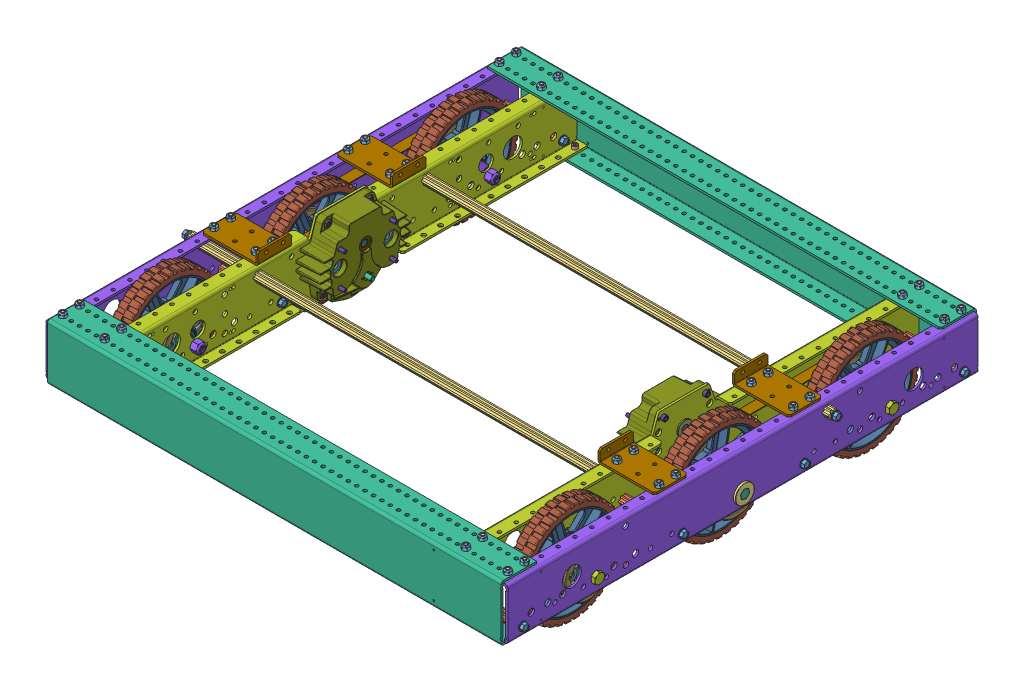
SolidWorks assembly 0 AM14U3 Full Square Drive Base, configuration Default. Lengths in mm.
Overall size (735.08 197.16 719.07).
302 component instances, 35 part files, 0 mates.
Components (placement in the parent):
- AM14U3 Square Half-1: AM14U3 Square Half [Default] at (-83.3124 74.3045 8.4761) size (722.96 197.16 715.14) (flexible)
  - AM14U3 Square Frame Half-1: AM14U3 Square Frame Half [Default] at (326.068 37.2757 -291.2758) size (722.38 116.33 715.14)
    - ThreadRollingScrew_0.25-20x0.75_FHTS 0.25-20-G-0.75-C-1: ThreadRollingScrew_0.25-20x0.75_FHTS 0.25-20-G-0.75-C [Default] at (-600.075 -67.691 639.064) x (-1 0 0) z (0 0.924225 0.381849) size (24.64 12.19 12.19)
    - ThreadRollingScrew_0.25-20x0.75_FHTS 0.25-20-G-0.75-C-2: ThreadRollingScrew_0.25-20x0.75_FHTS 0.25-20-G-0.75-C [Default] at (-600.075 -67.691 -27.94) x (-1 0 0) z (0 0.924225 0.381849) size (24.64 12.19 12.19)
    - ThreadRollingScrew_0.25-20x0.75_FHTS 0.25-20-G-0.75-C-3: ThreadRollingScrew_0.25-20x0.75_FHTS 0.25-20-G-0.75-C [Default] at (-692.15 -67.691 -27.813) size (24.64 12.19 12.19)
    - ThreadRollingScrew_0.25-20x0.75_FHTS 0.25-20-G-0.75-C-4: ThreadRollingScrew_0.25-20x0.75_FHTS 0.25-20-G-0.75-C [Default] at (-603.25 -15.494 178.562) size (24.64 12.19 12.19)
    - ThreadRollingScrew_0.25-20x0.75_FHTS 0.25-20-G-0.75-C-5: ThreadRollingScrew_0.25-20x0.75_FHTS 0.25-20-G-0.75-C [Default] at (-692.15 -67.691 638.937) size (24.64 12.19 12.19)
    - ThreadRollingScrew_0.25-20x0.75_FHTS 0.25-20-G-0.75-C-6: ThreadRollingScrew_0.25-20x0.75_FHTS 0.25-20-G-0.75-C [Default] at (19.05 -15.494 178.562) x (-1 0 0) z (0 0.525103 -0.851039) size (24.64 12.19 12.19)
    - 500Churro_3.375-1: 500Churro_3.375 [Default] at (-603.25 -67.691 -27.813) x (0 -0.866025 0.5) z (-1 0 0) size (14.66 12.7 85.72)
    - 500Churro_3.375-2: 500Churro_3.375 [Default] at (-603.25 -67.691 638.937) x (0 -0.866025 0.5) z (-1 0 0) size (14.66 12.7 85.72)
    - 500Churro_24.25-1: 500Churro_24.25 [Default] at (15.875 -15.494 178.562) x (0 0 -1) z (-1 0 0) size (14.66 12.7 615.95)
    - Screw_SHCS_10-32x0.5_HX-SHCS 0.19-32x1.375x1-C-1: Screw_SHCS_10-32x0.5_HX-SHCS 0.19-32x1.375x1-C [Default] at (-679.45 -11.43 -11.938) x (0 1 0) z (-0.440454 0 0.897775) size (17.53 7.94 7.94)
    - Screw_SHCS_10-32x0.5_HX-SHCS 0.19-32x1.375x1-C-2: Screw_SHCS_10-32x0.5_HX-SHCS 0.19-32x1.375x1-C [Default] at (-679.45 -11.43 -37.338) x (0 1 0) z (-0.063425 0 0.997987) size (17.53 7.94 7.94)
    - Screw_SHCS_10-32x0.5_HX-SHCS 0.19-32x1.375x1-C-3: Screw_SHCS_10-32x0.5_HX-SHCS 0.19-32x1.375x1-C [Default] at (-615.95 -11.43 -37.338) x (0 1 0) z (0 0 1) size (17.53 7.94 7.94)
    - Screw_SHCS_10-32x0.5_HX-SHCS 0.19-32x1.375x1-C-4: Screw_SHCS_10-32x0.5_HX-SHCS 0.19-32x1.375x1-C [Default] at (-615.95 -11.43 -11.938) x (0 1 0) z (0 0 1) size (17.53 7.94 7.94)
    - Screw_SHCS_10-32x0.5_HX-SHCS 0.19-32x1.375x1-C-5: Screw_SHCS_10-32x0.5_HX-SHCS 0.19-32x1.375x1-C [Default] at (-590.55 -73.152 -37.338) x (0 -1 0) z (0 0 1) size (17.53 7.94 7.94)
    - Screw_SHCS_10-32x0.5_HX-SHCS 0.19-32x1.375x1-C-6: Screw_SHCS_10-32x0.5_HX-SHCS 0.19-32x1.375x1-C [Default] at (-6.35 -11.176 -37.338) x (0 1 0) z (0.222581 0 0.974914) size (17.53 7.94 7.94)
    - Screw_SHCS_10-32x0.5_HX-SHCS 0.19-32x1.375x1-C-7: Screw_SHCS_10-32x0.5_HX-SHCS 0.19-32x1.375x1-C [Default] at (-6.35 -11.176 -11.938) x (0 1 0) z (0.81526 0 0.579096) size (17.53 7.94 7.94)
    - Screw_SHCS_10-32x0.5_HX-SHCS 0.19-32x1.375x1-C-8: Screw_SHCS_10-32x0.5_HX-SHCS 0.19-32x1.375x1-C [Default] at (-69.85 -11.176 -37.338) x (0 1 0) z (0 0 1) size (17.53 7.94 7.94)
    - Screw_SHCS_10-32x0.5_HX-SHCS 0.19-32x1.375x1-C-9: Screw_SHCS_10-32x0.5_HX-SHCS 0.19-32x1.375x1-C [Default] at (-69.85 -11.176 -11.938) x (0 1 0) z (0.111454 0 0.99377) size (17.53 7.94 7.94)
    - Screw_SHCS_10-32x0.5_HX-SHCS 0.19-32x1.375x1-C-10: Screw_SHCS_10-32x0.5_HX-SHCS 0.19-32x1.375x1-C [Default] at (-95.25 -73.406 -37.338) x (0 -1 0) z (0.007214 0 0.999974) size (17.53 7.94 7.94)
    - 10-32 Nylock Nut-1: 10-32 Nylock Nut [Default] at (-679.45 0 -37.338) x (1 0 0) z (0 1 0) size (9.53 11 5.96)
    - 10-32 Nylock Nut-2: 10-32 Nylock Nut [Default] at (-679.45 0 -11.938) x (0.114693 0 0.993401) z (0 1 0) size (9.53 11 5.96)
    - 10-32 Nylock Nut-3: 10-32 Nylock Nut [Default] at (-615.95 0 -11.938) x (1 0 0) z (0 1 0) size (9.53 11 5.96)
    - 10-32 Nylock Nut-4: 10-32 Nylock Nut [Default] at (-615.95 0 -37.338) x (1 0 0) z (0 1 0) size (9.53 11 5.96)
    - 10-32 Nylock Nut-5: 10-32 Nylock Nut [Default] at (-69.85 0 -11.938) x (1 0 0) z (0 1 0) size (9.53 11 5.96)
    - 10-32 Nylock Nut-6: 10-32 Nylock Nut [Default] at (-69.85 0 -37.338) x (1 0 0) z (0 1 0) size (9.53 11 5.96)
    - 10-32 Nylock Nut-7: 10-32 Nylock Nut [Default] at (-6.35 0 -11.938) x (1 0 0) z (0 1 0) size (9.53 11 5.96)
    - 10-32 Nylock Nut-8: 10-32 Nylock Nut [Default] at (-6.35 0 -37.338) x (1 0 0) z (0 1 0) size (9.53 11 5.96)
    - 10-32 Nylock Nut-9: 10-32 Nylock Nut [Default] at (-95.25 -84.582 -37.338) x (1 0 0) z (0 -1 0) size (9.53 11 5.96)
    - 10-32 Nylock Nut-10: 10-32 Nylock Nut [Default] at (-590.55 -84.582 -37.338) x (1 0 0) z (0 -1 0) size (9.53 11 5.96)
    - Screw_SHCS_10-32x0.5_HX-SHCS 0.19-32x1.375x1-C-11: Screw_SHCS_10-32x0.5_HX-SHCS 0.19-32x1.375x1-C [Default] at (-679.45 -11.43 191.262) x (0 1 0) z (0 0 1) size (17.53 7.94 7.94)
    - Screw_SHCS_10-32x0.5_HX-SHCS 0.19-32x1.375x1-C-12: Screw_SHCS_10-32x0.5_HX-SHCS 0.19-32x1.375x1-C [Default] at (-679.45 -11.43 216.662) x (0 1 0) z (0 0 1) size (17.53 7.94 7.94)
    - Screw_SHCS_10-32x0.5_HX-SHCS 0.19-32x1.375x1-C-13: Screw_SHCS_10-32x0.5_HX-SHCS 0.19-32x1.375x1-C [Default] at (-615.95 -11.43 191.262) x (0 1 0) z (0 0 1) size (17.53 7.94 7.94)
    - Screw_SHCS_10-32x0.5_HX-SHCS 0.19-32x1.375x1-C-14: Screw_SHCS_10-32x0.5_HX-SHCS 0.19-32x1.375x1-C [Default] at (-615.95 -11.43 216.662) x (0 1 0) z (0 0 1) size (17.53 7.94 7.94)
    - Screw_SHCS_10-32x0.5_HX-SHCS 0.19-32x1.375x1-C-15: Screw_SHCS_10-32x0.5_HX-SHCS 0.19-32x1.375x1-C [Default] at (-615.95 -11.43 394.462) x (0 1 0) z (0 0 1) size (17.53 7.94 7.94)
    - Screw_SHCS_10-32x0.5_HX-SHCS 0.19-32x1.375x1-C-16: Screw_SHCS_10-32x0.5_HX-SHCS 0.19-32x1.375x1-C [Default] at (-615.95 -11.43 419.862) x (0 1 0) z (0 0 1) size (17.53 7.94 7.94)
    - Screw_SHCS_10-32x0.5_HX-SHCS 0.19-32x1.375x1-C-17: Screw_SHCS_10-32x0.5_HX-SHCS 0.19-32x1.375x1-C [Default] at (-679.45 -11.43 394.462) x (0 1 0) z (0 0 1) size (17.53 7.94 7.94)
    - Screw_SHCS_10-32x0.5_HX-SHCS 0.19-32x1.375x1-C-18: Screw_SHCS_10-32x0.5_HX-SHCS 0.19-32x1.375x1-C [Default] at (-679.45 -11.43 419.862) x (0 1 0) z (0 0 1) size (17.53 7.94 7.94)
    - 10-32 Nylock Nut-11: 10-32 Nylock Nut [Default] at (-679.45 -0.254 419.862) x (1 0 0) z (0 1 0) size (9.53 11 5.96)
    - 10-32 Nylock Nut-12: 10-32 Nylock Nut [Default] at (-679.45 -0.254 394.462) x (1 0 0) z (0 1 0) size (9.53 11 5.96)
    - 10-32 Nylock Nut-13: 10-32 Nylock Nut [Default] at (-615.95 -0.254 394.462) x (1 0 0) z (0 1 0) size (9.53 11 5.96)
    - 10-32 Nylock Nut-14: 10-32 Nylock Nut [Default] at (-615.95 -0.254 419.862) x (1 0 0) z (0 1 0) size (9.53 11 5.96)
    - 10-32 Nylock Nut-15: 10-32 Nylock Nut [Default] at (-679.45 -0.254 216.662) x (1 0 0) z (0 1 0) size (9.53 11 5.96)
    - 10-32 Nylock Nut-16: 10-32 Nylock Nut [Default] at (-679.45 -0.254 191.262) x (1 0 0) z (0 1 0) size (9.53 11 5.96)
    - 10-32 Nylock Nut-17: 10-32 Nylock Nut [Default] at (-615.95 -0.254 216.662) x (1 0 0) z (0 1 0) size (9.53 11 5.96)
    - 10-32 Nylock Nut-18: 10-32 Nylock Nut [Default] at (-615.95 -0.254 191.262) x (1 0 0) z (0 1 0) size (9.53 11 5.96)
    - AM14U3EndPlate_Square-1: AM14U3EndPlate_Square [Default] at (-787.4 -81.407 -53.975) x (1 0 0) z (0 -1 0) size (685.8 53.98 84.58)
    - AM14U3InnerPlate_Square-1: AM14U3InnerPlate_Square [Default] at (-603.25 -77.216 711.962) x (0 0 -1) z (0 -1 0) size (711.2 38.1 116.33)
    - AM14U3OuterPlate_Square-1: AM14U3OuterPlate_Square [Default] at (-667.7485 -27.0221 21.6115) x (0 0 1) z (0 -1 0) size (711.2 19.05 77.72)
    - Bracket_2x3-1: Bracket_2x3 [Default] at (-685.8 -3.429 445.262) size (85.72 19.05 50.8)
    - Bracket_2x3-2: Bracket_2x3 [Default] at (-685.8 -3.429 242.062) size (85.72 19.05 50.8)
    - 500Churro_3.375-3: 500Churro_3.375 [Default] at (-688.975 -66.929 397.637) x (0 0.428755 -0.903421) z (1 0 0) size (14.66 12.7 85.72)
    - 500Churro_3.375-4: 500Churro_3.375 [Default] at (-688.975 -66.929 213.487) x (0 0 -1) z (1 0 0) size (14.66 12.7 85.72)
    - ThreadRollingScrew_0.25-20x0.75_FHTS 0.25-20-G-0.75-C-7: ThreadRollingScrew_0.25-20x0.75_FHTS 0.25-20-G-0.75-C [Default] at (-600.075 -66.929 397.637) x (-1 0 0) z (0 0.924225 0.381849) size (24.64 12.19 12.19)
    - ThreadRollingScrew_0.25-20x0.75_FHTS 0.25-20-G-0.75-C-8: ThreadRollingScrew_0.25-20x0.75_FHTS 0.25-20-G-0.75-C [Default] at (-600.075 -66.929 213.487) x (-1 0 0) z (0 0.924225 0.381849) size (24.64 12.19 12.19)
    - ThreadRollingScrew_0.25-20x0.75_FHTS 0.25-20-G-0.75-C-9: ThreadRollingScrew_0.25-20x0.75_FHTS 0.25-20-G-0.75-C [Default] at (-692.15 -66.929 397.637) x (1 0 0) z (0 -0.467404 -0.884044) size (24.64 12.19 12.19)
    - ThreadRollingScrew_0.25-20x0.75_FHTS 0.25-20-G-0.75-C-10: ThreadRollingScrew_0.25-20x0.75_FHTS 0.25-20-G-0.75-C [Default] at (-692.15 -66.929 213.487) size (24.64 12.19 12.19)
  - ToughboxMini-1: ToughboxMini [Default] at (-324.5487 -32.7384 105.387) x (0 0.001296 0.999999) z (-1 0 0) size (140.05 127.01 142.29)
    - TBMiniSmallHexShaft-1: TBMiniSmallHexShaft [Default] at (-129.7894 33.1737 -52.3959) x (-0.674239 -0.738513 0) z (-0.738513 0.674239 0) size (11 38.23 9.52)
    - LargeClusterGear_Hex_50t0.375-1: LargeClusterGear_Hex_50t0.375 [Default] at (-91.0349 50.9043 -67.5597) x (-0.674239 -0.738513 0) z (0 0 -1) size (65.97 66.04 10.34)
    - Bearing_FR6ZZ-1: Bearing_FR6ZZ [Default] at (-96.247 60.278 -52.5991) x (-0.893862 0.448342 0) z (0 0 1) size (24.69 24.69 7.16)
    - NylockNut_10-32-1: NylockNut_10-32 [Default] at (-129.8464 -8.0737 -56.3837) x (0.501678 0.865055 0) z (0 0 -1) size (9.53 11 5.96)
    - NylockNut_10-32-2: NylockNut_10-32 [Default] at (-59.2462 80.7349 -56.3837) x (0.999999 -0.001296 0) z (0 0 -1) size (9.53 11 5.96)
    - NylockNut_10-32-3: NylockNut_10-32 [Default] at (-122.7461 80.8172 -56.3837) x (0.500567 0.865698 0) z (0 0 -1) size (9.53 11 5.96)
    - NylockNut_10-32-4: NylockNut_10-32 [Default] at (-52.3764 -8.1741 -56.3837) x (-0.501678 -0.865055 0) z (0 0 -1) size (9.53 11 5.96)
    - Washer_5-16-1: Washer_5-16 [Default] at (-52.3162 38.3079 -77.7705) x (-0.418041 0.908428 0) z (0 0 -1) size (17.53 17.53 1.47)
    - Washer_5-16-2: Washer_5-16 [Default] at (-52.3162 38.3079 -76.2973) x (0.897267 -0.441488 0) z (0 0 -1) size (17.53 17.53 1.47)
    - Washer_5-16-3: Washer_5-16 [Default] at (-129.7861 38.4083 -77.7705) x (-0.990116 0.140253 0) z (0 0 1) size (17.53 17.53 1.47)
    - Washer_5-16-4: Washer_5-16 [Default] at (-129.7861 38.4083 -79.2437) x (-0.681761 0.731575 0) z (0 0 1) size (17.53 17.53 1.47)
    - CIMGear_14t8mm-1: CIMGear_14t8mm [Default] at (-52.3162 38.3079 -63.5973) x (-0.082762 0.996569 0) z (0 0 -1) size (20.03 20.32 12.7)
    - CIMGear_14t8mm-2: CIMGear_14t8mm [Default] at (-129.7861 38.4083 -63.5973) x (0.603285 0.797525 0) z (0 0 -1) size (20.03 20.32 12.7)
    - TBMiniHousing-1: TBMiniHousing [Default] at (-91.0876 10.1882 -86.3557) x (0.999999 -0.001296 0) z (0 0 1) size (139.9 118.55 41.62)
    - Screw_SHCS_10-32x0.625-1: Screw_SHCS_10-32x0.625 [Default] at (-52.2832 63.7078 -74.4685) x (-0.564778 -0.825243 0) z (-0.825243 0.564778 0) size (7.82 20.65 7.82)
    - Screw_SHCS_10-32x0.625-2: Screw_SHCS_10-32x0.625 [Default] at (-122.7461 80.8172 -42.5915) x (0.507484 -0.861661 0) z (-0.861661 -0.507484 0) size (7.82 20.65 7.82)
    - Screw_SHCS_10-32x0.625-3: Screw_SHCS_10-32x0.625 [Default] at (-52.3764 -8.1741 -42.5915) x (0.507484 -0.861661 0) z (-0.861661 -0.507484 0) size (7.82 20.65 7.82)
    - Screw_SHCS_10-32x0.625-4: Screw_SHCS_10-32x0.625 [Default] at (-129.8464 -8.0737 -42.5915) x (0.507484 -0.861661 0) z (-0.861661 -0.507484 0) size (7.82 20.65 7.82)
    - Screw_SHCS_10-32x0.625-5: Screw_SHCS_10-32x0.625 [Default] at (-59.2462 80.7349 -42.5915) x (0.740711 -0.671824 0) z (-0.671824 -0.740711 0) size (7.82 20.65 7.82)
    - Screw_SHCS_10-32x0.625-6: Screw_SHCS_10-32x0.625 [Default] at (-52.3491 12.9079 -74.4685) x (-0.564778 -0.825243 0) z (-0.825243 0.564778 0) size (7.82 20.65 7.82)
    - Screw_SHCS_10-32x0.625-7: Screw_SHCS_10-32x0.625 [Default] at (-129.7532 63.8083 -74.4685) x (-0.966277 -0.257503 0) z (-0.257503 0.966277 0) size (7.82 20.65 7.82)
    - Screw_SHCS_10-32x0.625-8: Screw_SHCS_10-32x0.625 [Default] at (-129.819 13.0083 -74.4685) x (-0.99652 0.083357 0) z (0.083357 0.99652 0) size (7.82 20.65 7.82)
    - Bearing_R6ZZ-1: Bearing_R6ZZ [Default] at (-91.0349 50.9043 -84.8317) x (0.958138 -0.286306 0) z (0 0 1) size (22.23 22.23 7.11)
    - Bearing_R6ZZ-2: Bearing_R6ZZ [Default] at (-91.0876 10.1882 -84.8317) x (-0.661529 0.74992 0) z (0 0 1) size (22.23 22.23 7.11)
    - RetainingClip-1: RetainingClip [Default] at (-129.7861 38.4083 -63.5973) x (0 0 1) z (-1 0 0) size (1.12 14.83 14.83)
    - RetainingClip-2: RetainingClip [Default] at (-52.3162 38.3079 -63.5973) x (0 0 1) z (-1 0 0) size (1.12 14.83 14.83)
    - ExternalKlipring-1: ExternalKlipring [Default] at (-91.0876 10.1882 -64.4355) x (0.996411 -0.084651 0) z (0 0 1) size (19.07 20.96 1.27)
    - Bearing_Hex_FR8ZZ-1: Bearing_Hex_FR8ZZ [Default] at (-91.0876 10.1882 -44.6717) x (0.73373 0.679441 0) z (0 0 -1) size (31.12 31.12 7.93)
    - SmallClusterGear_Hex_16t0.375-1: SmallClusterGear_Hex_16t0.375 [Default] at (-91.0349 50.9043 -67.5597) x (0 0 1) z (0.302452 -0.953165 0) size (15.19 22.57 22.57)
    - LargeOutputGear_Hex_48t0.5-1: LargeOutputGear_Hex_48t0.5 [Default] at (-91.0876 10.1882 -63.1655) x (0 0 1) z (-0.955278 0.295708 0) size (10.21 63.42 63.42)
    - TBMiniHexOutputShaft-1: TBMiniHexOutputShaft [Default] at (-51.6549 23.9851 -52.3197) x (0.73373 0.679441 0) z (0.679441 -0.73373 0) size (14.66 142.29 12.7)
  - Bearing_Hex_FR8ZZ-1: Bearing_Hex_FR8ZZ [Default] at (-369.3104 -22.6683 14.2862) x (0 -0.974861 0.222813) z (1 0 0) size (31.12 31.12 7.93)
  - hex finished bolt_ai_HFBOLT 0.375-16x2.5x1-C-1: hex finished bolt_ai_HFBOLT 0.375-16x2.5x1-C [Default] at (-372.2542 -20.8903 236.8339) size (69.67 16.48 14.27)
  - hex finished bolt_ai_HFBOLT 0.375-16x2.5x1-C-2: hex finished bolt_ai_HFBOLT 0.375-16x2.5x1-C [Default] at (-372.2542 -20.8903 -208.2615) size (69.67 16.48 14.27)
  - NylockNut_0.375-16_91831A127-1: NylockNut_0.375-16_91831A127 [Default] at (-274.007 -20.8903 236.8339) x (0 -1 0) z (0 0 1) size (14.29 12 16.5)
  - NylockNut_0.375-16_91831A127-2: NylockNut_0.375-16_91831A127 [Default] at (-274.007 -20.8903 -208.2615) x (0 -1 0) z (0 0 1) size (14.29 12 16.5)
  - Belt_15mm_Square-1: Belt_15mm_Square [Default] at (-289.0679 -20.8903 236.8339) x (0 -0.007989 -0.999968) z (-1 0 0) size (291.74 69.19 15)
  - Belt_15mm_Square-2: Belt_15mm_Square [Default] at (-335.856 -20.8903 -208.2615) x (0 -0.007989 0.999968) z (-1 0 0) size (291.74 69.19 15)
  - 6 HiGrip with hub and double pulley-1: 6 HiGrip with hub and double pulley [Default] at (-288.8079 -118.3384 -105.2016) x (-1 0 0) z (0 0.932481 0.36122) size (80.63 152.4 152.4)
    - 6 HiGrip Wheel Assembly Rev II-1: 6 HiGrip Wheel Assembly Rev II [Default] at (83.7987 67.439 110.9939) size (34.93 152.4 152.4)
      - 6 wheel Rev 4-1: 6 wheel Rev 4 [Default] at (-52.6446 9.4231 21.378) size (34.93 132.08 132.08)
      - 6 wheel tread II-1: 6 wheel tread II [Default] at (-65.3446 9.4231 21.378) x (0 0 -1) z (1 0 0) size (152.4 152.4 25.58)
    - HalfPulley_42t5mm-1: HalfPulley_42t5mm [Default] at (47.6006 76.862 132.3719) x (1 0 0) z (0 -0.5 0.866025) size (13 74.23 74.23)
    - HalfPulley_42t5mm-2: HalfPulley_42t5mm [Default] at (64.263 76.862 132.3719) x (-1 0 0) z (0 -0.499927 0.866067) size (13 74.23 74.23)
    - Washer_5-16-1: Washer_5-16 [Default] at (63.247 76.8605 108.5602) x (0 -0.812665 -0.582732) z (1 0 0) size (17.53 17.53 1.47)
    - Washer_5-16-2: Washer_5-16 [Default] at (63.247 97.4833 120.4656) x (0 0.998209 0.059825) z (1 0 0) size (17.53 17.53 1.47)
    - Washer_5-16-3: Washer_5-16 [Default] at (63.247 56.2398 144.2799) x (0 -0.026074 -0.99966) z (1 0 0) size (17.53 17.53 1.47)
    - Washer_5-16-4: Washer_5-16 [Default] at (63.247 76.8625 156.1852) x (0 -0.766208 -0.642593) z (1 0 0) size (17.53 17.53 1.47)
    - Washer_5-16-5: Washer_5-16 [Default] at (63.247 97.4843 144.2781) x (0 -0.833184 -0.552996) z (1 0 0) size (17.53 17.53 1.47)
    - Washer_5-16-6: Washer_5-16 [Default] at (63.247 56.2388 120.4674) x (0 -0.998572 0.053424) z (1 0 0) size (17.53 17.53 1.47)
    - HalfPulley_42t5mm-3: HalfPulley_42t5mm [Default] at (-1.9548 76.8628 132.3714) x (1 0 0) z (0 -1 -0.000063) size (13 74.23 74.23)
    - HalfPulley_42t5mm-4: HalfPulley_42t5mm [Default] at (14.7076 76.8628 132.3714) x (-1 0 0) z (0 -1 0.000021) size (13 74.23 74.23)
    - HexHub_500EX-1: HexHub_500EX [Default] at (-8.3048 76.862 132.3719) x (0 -0.866025 -0.5) z (0 -0.5 0.866025) size (55.37 25.4 51.33)
    - Washer_5-16-7: Washer_5-16 [Default] at (-5.2568 97.4843 120.4656) x (0 0.577286 0.816542) z (-1 0 0) size (17.53 17.53 1.47)
    - Washer_5-16-8: Washer_5-16 [Default] at (-5.2568 76.862 108.5594) x (0 0.877244 0.480045) z (-1 0 0) size (17.53 17.53 1.47)
    - Washer_5-16-9: Washer_5-16 [Default] at (-5.2568 56.2398 120.4656) x (0 -0.894136 -0.447796) z (-1 0 0) size (17.53 17.53 1.47)
    - Washer_5-16-10: Washer_5-16 [Default] at (-5.2568 97.4843 144.2781) x (0 -0.559623 -0.828747) z (-1 0 0) size (17.53 17.53 1.47)
    - Washer_5-16-11: Washer_5-16 [Default] at (-5.2568 56.2398 144.2781) x (0 -0.82184 -0.569719) z (-1 0 0) size (17.53 17.53 1.47)
    - Washer_5-16-12: Washer_5-16 [Default] at (-5.2568 76.862 156.1844) x (0 -0.981812 0.189856) z (-1 0 0) size (17.53 17.53 1.47)
    - Spacer_Hex_0.57x0.5-1: Spacer_Hex_0.57x0.5 [Default] at (57.8495 76.862 132.3719) x (0 -0.866025 -0.5) z (0 -0.5 0.866025) size (28.55 14.48 28.55)
  - 6 HiGrip with bearings, pulleys and spacers_2-1: 6 HiGrip with bearings, pulleys and spacers_2 [Default] at (-287.4242 128.7008 -175.8179) x (-1 0 0) z (0 -0.951569 0.307436) size (85.56 152.4 152.4)
    - 6 HiGrip Wheel Assembly Rev II-1: 6 HiGrip Wheel Assembly Rev II [Default] at (83.7987 67.439 110.9939) size (34.93 152.4 152.4)
      - 6 wheel Rev 4-1: 6 wheel Rev 4 [Default] at (-52.6446 9.4231 21.378) size (34.93 132.08 132.08)
      - 6 wheel tread II-1: 6 wheel tread II [Default] at (-65.3446 9.4231 21.378) x (0 0 -1) z (1 0 0) size (152.4 152.4 25.58)
    - HalfPulley_42t5mm-1: HalfPulley_42t5mm [Default] at (47.6006 76.862 132.3719) x (1 0 0) z (0 -0.5 0.866025) size (13 74.23 74.23)
    - HalfPulley_42t5mm-2: HalfPulley_42t5mm [Default] at (64.263 76.862 132.3719) x (-1 0 0) z (0 -0.499927 0.866067) size (13 74.23 74.23)
    - Bearing_1614ZZ-1: Bearing_1614ZZ [Default] at (62.612 76.862 132.3719) x (0 -0.157148 -0.987575) z (-1 0 0) size (28.58 28.58 9.53)
    - Bearing_1614ZZ-2: Bearing_1614ZZ [Default] at (15.2791 76.862 132.3719) x (0 0 -1) z (1 0 0) size (28.58 28.58 9.53)
    - Washer_5-16-1: Washer_5-16 [Default] at (63.247 76.8605 108.5602) x (0 0.946124 0.323805) z (1 0 0) size (17.53 17.53 1.47)
    - Washer_5-16-2: Washer_5-16 [Default] at (63.247 97.4833 120.4656) x (0 0.770474 -0.637472) z (1 0 0) size (17.53 17.53 1.47)
    - Washer_5-16-3: Washer_5-16 [Default] at (63.247 56.2398 144.2799) x (0 0 -1) z (1 0 0) size (17.53 17.53 1.47)
    - Washer_5-16-4: Washer_5-16 [Default] at (63.247 76.8625 156.1852) x (0 -0.95788 -0.287168) z (1 0 0) size (17.53 17.53 1.47)
    - Washer_5-16-5: Washer_5-16 [Default] at (63.247 97.4843 144.2781) x (0 -0.653102 0.75727) z (1 0 0) size (17.53 17.53 1.47)
    - Washer_5-16-6: Washer_5-16 [Default] at (63.247 56.2388 120.4674) x (0 -0.977348 -0.211637) z (1 0 0) size (17.53 17.53 1.47)
    - Spacer_0.28x0.382-1: Spacer_0.28x0.382 [Default] at (74.4865 76.862 132.3719) x (0 -0.35357 0.935408) z (-1 0 0) size (13.16 13.16 7.11)
    - Spacer_0.85x0.38-1: Spacer_0.85x0.38 [Default] at (-11.0734 76.862 132.3719) x (0 0 -1) z (1 0 0) size (19.05 19.05 21.59)
  - 6 HiGrip with bearings, pulleys and spacers_2-2: 6 HiGrip with bearings, pulleys and spacers_2 [Default] at (-352.4997 -117.9713 118.4896) x (1 0 0) z (0 0.160247 0.987077) size (85.56 152.4 152.4)
    - 6 HiGrip Wheel Assembly Rev II-1: 6 HiGrip Wheel Assembly Rev II [Default] at (83.7987 67.439 110.9939) size (34.93 152.4 152.4)
      - 6 wheel Rev 4-1: 6 wheel Rev 4 [Default] at (-52.6446 9.4231 21.378) size (34.93 132.08 132.08)
      - 6 wheel tread II-1: 6 wheel tread II [Default] at (-65.3446 9.4231 21.378) x (0 0 -1) z (1 0 0) size (152.4 152.4 25.58)
    - HalfPulley_42t5mm-1: HalfPulley_42t5mm [Default] at (47.6006 76.862 132.3719) x (1 0 0) z (0 -0.5 0.866025) size (13 74.23 74.23)
    - HalfPulley_42t5mm-2: HalfPulley_42t5mm [Default] at (64.263 76.862 132.3719) x (-1 0 0) z (0 -0.499927 0.866067) size (13 74.23 74.23)
    - Bearing_1614ZZ-1: Bearing_1614ZZ [Default] at (62.612 76.862 132.3719) x (0 -0.157148 -0.987575) z (-1 0 0) size (28.58 28.58 9.53)
    - Bearing_1614ZZ-2: Bearing_1614ZZ [Default] at (15.2791 76.862 132.3719) x (0 0 -1) z (1 0 0) size (28.58 28.58 9.53)
    - Washer_5-16-1: Washer_5-16 [Default] at (63.247 76.8605 108.5602) x (0 0.946124 0.323805) z (1 0 0) size (17.53 17.53 1.47)
    - Washer_5-16-2: Washer_5-16 [Default] at (63.247 97.4833 120.4656) x (0 0.770474 -0.637472) z (1 0 0) size (17.53 17.53 1.47)
    - Washer_5-16-3: Washer_5-16 [Default] at (63.247 56.2398 144.2799) x (0 0 -1) z (1 0 0) size (17.53 17.53 1.47)
    - Washer_5-16-4: Washer_5-16 [Default] at (63.247 76.8625 156.1852) x (0 -0.95788 -0.287168) z (1 0 0) size (17.53 17.53 1.47)
    - Washer_5-16-5: Washer_5-16 [Default] at (63.247 97.4843 144.2781) x (0 -0.653102 0.75727) z (1 0 0) size (17.53 17.53 1.47)
    - Washer_5-16-6: Washer_5-16 [Default] at (63.247 56.2388 120.4674) x (0 -0.977348 -0.211637) z (1 0 0) size (17.53 17.53 1.47)
    - Spacer_0.28x0.382-1: Spacer_0.28x0.382 [Default] at (74.4865 76.862 132.3719) x (0 -0.35357 0.935408) z (-1 0 0) size (13.16 13.16 7.11)
    - Spacer_0.85x0.38-1: Spacer_0.85x0.38 [Default] at (-11.0734 76.862 132.3719) x (0 0 -1) z (1 0 0) size (19.05 19.05 21.59)
- AM14U3 Square Half-2: AM14U3 Square Half [Default] at (-116.9765 74.3045 37.0485) x (-1 0 0) z (0 0 -1) size (722.96 193.43 715.14) (flexible)
  - AM14U3 Square Frame Half-1: AM14U3 Square Frame Half [Default] at (326.068 37.2757 -291.2758) size (722.38 116.33 715.14)
    - ThreadRollingScrew_0.25-20x0.75_FHTS 0.25-20-G-0.75-C-1: ThreadRollingScrew_0.25-20x0.75_FHTS 0.25-20-G-0.75-C [Default] at (-600.075 -67.691 639.064) x (-1 0 0) z (0 0.924225 0.381849) size (24.64 12.19 12.19)
    - ThreadRollingScrew_0.25-20x0.75_FHTS 0.25-20-G-0.75-C-2: ThreadRollingScrew_0.25-20x0.75_FHTS 0.25-20-G-0.75-C [Default] at (-600.075 -67.691 -27.94) x (-1 0 0) z (0 0.924225 0.381849) size (24.64 12.19 12.19)
    - ThreadRollingScrew_0.25-20x0.75_FHTS 0.25-20-G-0.75-C-3: ThreadRollingScrew_0.25-20x0.75_FHTS 0.25-20-G-0.75-C [Default] at (-692.15 -67.691 -27.813) size (24.64 12.19 12.19)
    - ThreadRollingScrew_0.25-20x0.75_FHTS 0.25-20-G-0.75-C-4: ThreadRollingScrew_0.25-20x0.75_FHTS 0.25-20-G-0.75-C [Default] at (-603.25 -15.494 178.562) size (24.64 12.19 12.19)
    - ThreadRollingScrew_0.25-20x0.75_FHTS 0.25-20-G-0.75-C-5: ThreadRollingScrew_0.25-20x0.75_FHTS 0.25-20-G-0.75-C [Default] at (-692.15 -67.691 638.937) size (24.64 12.19 12.19)
    - ThreadRollingScrew_0.25-20x0.75_FHTS 0.25-20-G-0.75-C-6: ThreadRollingScrew_0.25-20x0.75_FHTS 0.25-20-G-0.75-C [Default] at (19.05 -15.494 178.562) x (-1 0 0) z (0 0.525103 -0.851039) size (24.64 12.19 12.19)
    - 500Churro_3.375-1: 500Churro_3.375 [Default] at (-603.25 -67.691 -27.813) x (0 -0.866025 0.5) z (-1 0 0) size (14.66 12.7 85.72)
    - 500Churro_3.375-2: 500Churro_3.375 [Default] at (-603.25 -67.691 638.937) x (0 -0.866025 0.5) z (-1 0 0) size (14.66 12.7 85.72)
    - 500Churro_24.25-1: 500Churro_24.25 [Default] at (15.875 -15.494 178.562) x (0 0 -1) z (-1 0 0) size (14.66 12.7 615.95)
    - Screw_SHCS_10-32x0.5_HX-SHCS 0.19-32x1.375x1-C-1: Screw_SHCS_10-32x0.5_HX-SHCS 0.19-32x1.375x1-C [Default] at (-679.45 -11.43 -11.938) x (0 1 0) z (-0.440454 0 0.897775) size (17.53 7.94 7.94)
    - Screw_SHCS_10-32x0.5_HX-SHCS 0.19-32x1.375x1-C-2: Screw_SHCS_10-32x0.5_HX-SHCS 0.19-32x1.375x1-C [Default] at (-679.45 -11.43 -37.338) x (0 1 0) z (-0.063425 0 0.997987) size (17.53 7.94 7.94)
    - Screw_SHCS_10-32x0.5_HX-SHCS 0.19-32x1.375x1-C-3: Screw_SHCS_10-32x0.5_HX-SHCS 0.19-32x1.375x1-C [Default] at (-615.95 -11.43 -37.338) x (0 1 0) z (0 0 1) size (17.53 7.94 7.94)
    - Screw_SHCS_10-32x0.5_HX-SHCS 0.19-32x1.375x1-C-4: Screw_SHCS_10-32x0.5_HX-SHCS 0.19-32x1.375x1-C [Default] at (-615.95 -11.43 -11.938) x (0 1 0) z (0 0 1) size (17.53 7.94 7.94)
    - Screw_SHCS_10-32x0.5_HX-SHCS 0.19-32x1.375x1-C-5: Screw_SHCS_10-32x0.5_HX-SHCS 0.19-32x1.375x1-C [Default] at (-590.55 -73.152 -37.338) x (0 -1 0) z (0 0 1) size (17.53 7.94 7.94)
    - Screw_SHCS_10-32x0.5_HX-SHCS 0.19-32x1.375x1-C-6: Screw_SHCS_10-32x0.5_HX-SHCS 0.19-32x1.375x1-C [Default] at (-6.35 -11.176 -37.338) x (0 1 0) z (0.222581 0 0.974914) size (17.53 7.94 7.94)
    - Screw_SHCS_10-32x0.5_HX-SHCS 0.19-32x1.375x1-C-7: Screw_SHCS_10-32x0.5_HX-SHCS 0.19-32x1.375x1-C [Default] at (-6.35 -11.176 -11.938) x (0 1 0) z (0.81526 0 0.579096) size (17.53 7.94 7.94)
    - Screw_SHCS_10-32x0.5_HX-SHCS 0.19-32x1.375x1-C-8: Screw_SHCS_10-32x0.5_HX-SHCS 0.19-32x1.375x1-C [Default] at (-69.85 -11.176 -37.338) x (0 1 0) z (0 0 1) size (17.53 7.94 7.94)
    - Screw_SHCS_10-32x0.5_HX-SHCS 0.19-32x1.375x1-C-9: Screw_SHCS_10-32x0.5_HX-SHCS 0.19-32x1.375x1-C [Default] at (-69.85 -11.176 -11.938) x (0 1 0) z (0.111454 0 0.99377) size (17.53 7.94 7.94)
    - Screw_SHCS_10-32x0.5_HX-SHCS 0.19-32x1.375x1-C-10: Screw_SHCS_10-32x0.5_HX-SHCS 0.19-32x1.375x1-C [Default] at (-95.25 -73.406 -37.338) x (0 -1 0) z (0.007214 0 0.999974) size (17.53 7.94 7.94)
    - 10-32 Nylock Nut-1: 10-32 Nylock Nut [Default] at (-679.45 0 -37.338) x (1 0 0) z (0 1 0) size (9.53 11 5.96)
    - 10-32 Nylock Nut-2: 10-32 Nylock Nut [Default] at (-679.45 0 -11.938) x (0.114693 0 0.993401) z (0 1 0) size (9.53 11 5.96)
    - 10-32 Nylock Nut-3: 10-32 Nylock Nut [Default] at (-615.95 0 -11.938) x (1 0 0) z (0 1 0) size (9.53 11 5.96)
    - 10-32 Nylock Nut-4: 10-32 Nylock Nut [Default] at (-615.95 0 -37.338) x (1 0 0) z (0 1 0) size (9.53 11 5.96)
    - 10-32 Nylock Nut-5: 10-32 Nylock Nut [Default] at (-69.85 0 -11.938) x (1 0 0) z (0 1 0) size (9.53 11 5.96)
    - 10-32 Nylock Nut-6: 10-32 Nylock Nut [Default] at (-69.85 0 -37.338) x (1 0 0) z (0 1 0) size (9.53 11 5.96)
    - 10-32 Nylock Nut-7: 10-32 Nylock Nut [Default] at (-6.35 0 -11.938) x (1 0 0) z (0 1 0) size (9.53 11 5.96)
    - 10-32 Nylock Nut-8: 10-32 Nylock Nut [Default] at (-6.35 0 -37.338) x (1 0 0) z (0 1 0) size (9.53 11 5.96)
    - 10-32 Nylock Nut-9: 10-32 Nylock Nut [Default] at (-95.25 -84.582 -37.338) x (1 0 0) z (0 -1 0) size (9.53 11 5.96)
    - 10-32 Nylock Nut-10: 10-32 Nylock Nut [Default] at (-590.55 -84.582 -37.338) x (1 0 0) z (0 -1 0) size (9.53 11 5.96)
    - Screw_SHCS_10-32x0.5_HX-SHCS 0.19-32x1.375x1-C-11: Screw_SHCS_10-32x0.5_HX-SHCS 0.19-32x1.375x1-C [Default] at (-679.45 -11.43 191.262) x (0 1 0) z (0 0 1) size (17.53 7.94 7.94)
    - Screw_SHCS_10-32x0.5_HX-SHCS 0.19-32x1.375x1-C-12: Screw_SHCS_10-32x0.5_HX-SHCS 0.19-32x1.375x1-C [Default] at (-679.45 -11.43 216.662) x (0 1 0) z (0 0 1) size (17.53 7.94 7.94)
    - Screw_SHCS_10-32x0.5_HX-SHCS 0.19-32x1.375x1-C-13: Screw_SHCS_10-32x0.5_HX-SHCS 0.19-32x1.375x1-C [Default] at (-615.95 -11.43 191.262) x (0 1 0) z (0 0 1) size (17.53 7.94 7.94)
    - Screw_SHCS_10-32x0.5_HX-SHCS 0.19-32x1.375x1-C-14: Screw_SHCS_10-32x0.5_HX-SHCS 0.19-32x1.375x1-C [Default] at (-615.95 -11.43 216.662) x (0 1 0) z (0 0 1) size (17.53 7.94 7.94)
    - Screw_SHCS_10-32x0.5_HX-SHCS 0.19-32x1.375x1-C-15: Screw_SHCS_10-32x0.5_HX-SHCS 0.19-32x1.375x1-C [Default] at (-615.95 -11.43 394.462) x (0 1 0) z (0 0 1) size (17.53 7.94 7.94)
    - Screw_SHCS_10-32x0.5_HX-SHCS 0.19-32x1.375x1-C-16: Screw_SHCS_10-32x0.5_HX-SHCS 0.19-32x1.375x1-C [Default] at (-615.95 -11.43 419.862) x (0 1 0) z (0 0 1) size (17.53 7.94 7.94)
    - Screw_SHCS_10-32x0.5_HX-SHCS 0.19-32x1.375x1-C-17: Screw_SHCS_10-32x0.5_HX-SHCS 0.19-32x1.375x1-C [Default] at (-679.45 -11.43 394.462) x (0 1 0) z (0 0 1) size (17.53 7.94 7.94)
    - Screw_SHCS_10-32x0.5_HX-SHCS 0.19-32x1.375x1-C-18: Screw_SHCS_10-32x0.5_HX-SHCS 0.19-32x1.375x1-C [Default] at (-679.45 -11.43 419.862) x (0 1 0) z (0 0 1) size (17.53 7.94 7.94)
    - 10-32 Nylock Nut-11: 10-32 Nylock Nut [Default] at (-679.45 -0.254 419.862) x (1 0 0) z (0 1 0) size (9.53 11 5.96)
    - 10-32 Nylock Nut-12: 10-32 Nylock Nut [Default] at (-679.45 -0.254 394.462) x (1 0 0) z (0 1 0) size (9.53 11 5.96)
    - 10-32 Nylock Nut-13: 10-32 Nylock Nut [Default] at (-615.95 -0.254 394.462) x (1 0 0) z (0 1 0) size (9.53 11 5.96)
    - 10-32 Nylock Nut-14: 10-32 Nylock Nut [Default] at (-615.95 -0.254 419.862) x (1 0 0) z (0 1 0) size (9.53 11 5.96)
    - 10-32 Nylock Nut-15: 10-32 Nylock Nut [Default] at (-679.45 -0.254 216.662) x (1 0 0) z (0 1 0) size (9.53 11 5.96)
    - 10-32 Nylock Nut-16: 10-32 Nylock Nut [Default] at (-679.45 -0.254 191.262) x (1 0 0) z (0 1 0) size (9.53 11 5.96)
    - 10-32 Nylock Nut-17: 10-32 Nylock Nut [Default] at (-615.95 -0.254 216.662) x (1 0 0) z (0 1 0) size (9.53 11 5.96)
    - 10-32 Nylock Nut-18: 10-32 Nylock Nut [Default] at (-615.95 -0.254 191.262) x (1 0 0) z (0 1 0) size (9.53 11 5.96)
    - AM14U3EndPlate_Square-1: AM14U3EndPlate_Square [Default] at (-787.4 -81.407 -53.975) x (1 0 0) z (0 -1 0) size (685.8 53.98 84.58)
    - AM14U3InnerPlate_Square-1: AM14U3InnerPlate_Square [Default] at (-603.25 -77.216 711.962) x (0 0 -1) z (0 -1 0) size (711.2 38.1 116.33)
    - AM14U3OuterPlate_Square-1: AM14U3OuterPlate_Square [Default] at (-667.7485 -27.0221 21.6115) x (0 0 1) z (0 -1 0) size (711.2 19.05 77.72)
    - Bracket_2x3-1: Bracket_2x3 [Default] at (-685.8 -3.429 445.262) size (85.72 19.05 50.8)
    - Bracket_2x3-2: Bracket_2x3 [Default] at (-685.8 -3.429 242.062) size (85.72 19.05 50.8)
    - 500Churro_3.375-3: 500Churro_3.375 [Default] at (-688.975 -66.929 397.637) x (0 0.428755 -0.903421) z (1 0 0) size (14.66 12.7 85.72)
    - 500Churro_3.375-4: 500Churro_3.375 [Default] at (-688.975 -66.929 213.487) x (0 0 -1) z (1 0 0) size (14.66 12.7 85.72)
    - ThreadRollingScrew_0.25-20x0.75_FHTS 0.25-20-G-0.75-C-7: ThreadRollingScrew_0.25-20x0.75_FHTS 0.25-20-G-0.75-C [Default] at (-600.075 -66.929 397.637) x (-1 0 0) z (0 0.924225 0.381849) size (24.64 12.19 12.19)
    - ThreadRollingScrew_0.25-20x0.75_FHTS 0.25-20-G-0.75-C-8: ThreadRollingScrew_0.25-20x0.75_FHTS 0.25-20-G-0.75-C [Default] at (-600.075 -66.929 213.487) x (-1 0 0) z (0 0.924225 0.381849) size (24.64 12.19 12.19)
    - ThreadRollingScrew_0.25-20x0.75_FHTS 0.25-20-G-0.75-C-9: ThreadRollingScrew_0.25-20x0.75_FHTS 0.25-20-G-0.75-C [Default] at (-692.15 -66.929 397.637) x (1 0 0) z (0 -0.467404 -0.884044) size (24.64 12.19 12.19)
    - ThreadRollingScrew_0.25-20x0.75_FHTS 0.25-20-G-0.75-C-10: ThreadRollingScrew_0.25-20x0.75_FHTS 0.25-20-G-0.75-C [Default] at (-692.15 -66.929 213.487) size (24.64 12.19 12.19)
  - ToughboxMini-1: ToughboxMini [Default] at (-324.5487 -32.7384 105.387) x (0 0.001296 0.999999) z (-1 0 0) size (140.05 127.01 142.29)
    - TBMiniSmallHexShaft-1: TBMiniSmallHexShaft [Default] at (-129.7894 33.1737 -52.3959) x (-0.674239 -0.738513 0) z (-0.738513 0.674239 0) size (11 38.23 9.52)
    - LargeClusterGear_Hex_50t0.375-1: LargeClusterGear_Hex_50t0.375 [Default] at (-91.0349 50.9043 -67.5597) x (-0.674239 -0.738513 0) z (0 0 -1) size (65.97 66.04 10.34)
    - Bearing_FR6ZZ-1: Bearing_FR6ZZ [Default] at (-96.247 60.278 -52.5991) x (-0.893862 0.448342 0) z (0 0 1) size (24.69 24.69 7.16)
    - NylockNut_10-32-1: NylockNut_10-32 [Default] at (-129.8464 -8.0737 -56.3837) x (0.501678 0.865055 0) z (0 0 -1) size (9.53 11 5.96)
    - NylockNut_10-32-2: NylockNut_10-32 [Default] at (-59.2462 80.7349 -56.3837) x (0.999999 -0.001296 0) z (0 0 -1) size (9.53 11 5.96)
    - NylockNut_10-32-3: NylockNut_10-32 [Default] at (-122.7461 80.8172 -56.3837) x (0.500567 0.865698 0) z (0 0 -1) size (9.53 11 5.96)
    - NylockNut_10-32-4: NylockNut_10-32 [Default] at (-52.3764 -8.1741 -56.3837) x (-0.501678 -0.865055 0) z (0 0 -1) size (9.53 11 5.96)
    - Washer_5-16-1: Washer_5-16 [Default] at (-52.3162 38.3079 -77.7705) x (-0.418041 0.908428 0) z (0 0 -1) size (17.53 17.53 1.47)
    - Washer_5-16-2: Washer_5-16 [Default] at (-52.3162 38.3079 -76.2973) x (0.897267 -0.441488 0) z (0 0 -1) size (17.53 17.53 1.47)
    - Washer_5-16-3: Washer_5-16 [Default] at (-129.7861 38.4083 -77.7705) x (-0.990116 0.140253 0) z (0 0 1) size (17.53 17.53 1.47)
    - Washer_5-16-4: Washer_5-16 [Default] at (-129.7861 38.4083 -79.2437) x (-0.681761 0.731575 0) z (0 0 1) size (17.53 17.53 1.47)
    - CIMGear_14t8mm-1: CIMGear_14t8mm [Default] at (-52.3162 38.3079 -63.5973) x (-0.082762 0.996569 0) z (0 0 -1) size (20.03 20.32 12.7)
    - CIMGear_14t8mm-2: CIMGear_14t8mm [Default] at (-129.7861 38.4083 -63.5973) x (0.603285 0.797525 0) z (0 0 -1) size (20.03 20.32 12.7)
    - TBMiniHousing-1: TBMiniHousing [Default] at (-91.0876 10.1882 -86.3557) x (0.999999 -0.001296 0) z (0 0 1) size (139.9 118.55 41.62)
    - Screw_SHCS_10-32x0.625-1: Screw_SHCS_10-32x0.625 [Default] at (-52.2832 63.7078 -74.4685) x (-0.564778 -0.825243 0) z (-0.825243 0.564778 0) size (7.82 20.65 7.82)
    - Screw_SHCS_10-32x0.625-2: Screw_SHCS_10-32x0.625 [Default] at (-122.7461 80.8172 -42.5915) x (0.507484 -0.861661 0) z (-0.861661 -0.507484 0) size (7.82 20.65 7.82)
    - Screw_SHCS_10-32x0.625-3: Screw_SHCS_10-32x0.625 [Default] at (-52.3764 -8.1741 -42.5915) x (0.507484 -0.861661 0) z (-0.861661 -0.507484 0) size (7.82 20.65 7.82)
    - Screw_SHCS_10-32x0.625-4: Screw_SHCS_10-32x0.625 [Default] at (-129.8464 -8.0737 -42.5915) x (0.507484 -0.861661 0) z (-0.861661 -0.507484 0) size (7.82 20.65 7.82)
    - Screw_SHCS_10-32x0.625-5: Screw_SHCS_10-32x0.625 [Default] at (-59.2462 80.7349 -42.5915) x (0.740711 -0.671824 0) z (-0.671824 -0.740711 0) size (7.82 20.65 7.82)
    - Screw_SHCS_10-32x0.625-6: Screw_SHCS_10-32x0.625 [Default] at (-52.3491 12.9079 -74.4685) x (-0.564778 -0.825243 0) z (-0.825243 0.564778 0) size (7.82 20.65 7.82)
    - Screw_SHCS_10-32x0.625-7: Screw_SHCS_10-32x0.625 [Default] at (-129.7532 63.8083 -74.4685) x (-0.966277 -0.257503 0) z (-0.257503 0.966277 0) size (7.82 20.65 7.82)
    - Screw_SHCS_10-32x0.625-8: Screw_SHCS_10-32x0.625 [Default] at (-129.819 13.0083 -74.4685) x (-0.99652 0.083357 0) z (0.083357 0.99652 0) size (7.82 20.65 7.82)
    - Bearing_R6ZZ-1: Bearing_R6ZZ [Default] at (-91.0349 50.9043 -84.8317) x (0.958138 -0.286306 0) z (0 0 1) size (22.23 22.23 7.11)
    - Bearing_R6ZZ-2: Bearing_R6ZZ [Default] at (-91.0876 10.1882 -84.8317) x (-0.661529 0.74992 0) z (0 0 1) size (22.23 22.23 7.11)
    - RetainingClip-1: RetainingClip [Default] at (-129.7861 38.4083 -63.5973) x (0 0 1) z (-1 0 0) size (1.12 14.83 14.83)
    - RetainingClip-2: RetainingClip [Default] at (-52.3162 38.3079 -63.5973) x (0 0 1) z (-1 0 0) size (1.12 14.83 14.83)
    - ExternalKlipring-1: ExternalKlipring [Default] at (-91.0876 10.1882 -64.4355) x (0.996411 -0.084651 0) z (0 0 1) size (19.07 20.96 1.27)
    - Bearing_Hex_FR8ZZ-1: Bearing_Hex_FR8ZZ [Default] at (-91.0876 10.1882 -44.6717) x (0.73373 0.679441 0) z (0 0 -1) size (31.12 31.12 7.93)
    - SmallClusterGear_Hex_16t0.375-1: SmallClusterGear_Hex_16t0.375 [Default] at (-91.0349 50.9043 -67.5597) x (0 0 1) z (0.302452 -0.953165 0) size (15.19 22.57 22.57)
    - LargeOutputGear_Hex_48t0.5-1: LargeOutputGear_Hex_48t0.5 [Default] at (-91.0876 10.1882 -63.1655) x (0 0 1) z (-0.955278 0.295708 0) size (10.21 63.42 63.42)
    - TBMiniHexOutputShaft-1: TBMiniHexOutputShaft [Default] at (-51.6549 23.9851 -52.3197) x (0.73373 0.679441 0) z (0.679441 -0.73373 0) size (14.66 142.29 12.7)
  - Bearing_Hex_FR8ZZ-1: Bearing_Hex_FR8ZZ [Default] at (-369.3104 -22.6683 14.2862) x (0 -0.974861 0.222813) z (1 0 0) size (31.12 31.12 7.93)
  - hex finished bolt_ai_HFBOLT 0.375-16x2.5x1-C-1: hex finished bolt_ai_HFBOLT 0.375-16x2.5x1-C [Default] at (-372.2542 -20.8903 236.8339) size (69.67 16.48 14.27)
  - hex finished bolt_ai_HFBOLT 0.375-16x2.5x1-C-2: hex finished bolt_ai_HFBOLT 0.375-16x2.5x1-C [Default] at (-372.2542 -20.8903 -208.2615) size (69.67 16.48 14.27)
  - NylockNut_0.375-16_91831A127-1: NylockNut_0.375-16_91831A127 [Default] at (-274.007 -20.8903 236.8339) x (0 -1 0) z (0 0 1) size (14.29 12 16.5)
  - NylockNut_0.375-16_91831A127-2: NylockNut_0.375-16_91831A127 [Default] at (-274.007 -20.8903 -208.2615) x (0 -1 0) z (0 0 1) size (14.29 12 16.5)
  - Belt_15mm_Square-1: Belt_15mm_Square [Default] at (-289.0679 -20.8903 236.8339) x (0 -0.007989 -0.999968) z (-1 0 0) size (291.74 69.19 15)
  - Belt_15mm_Square-2: Belt_15mm_Square [Default] at (-335.856 -20.8903 -208.2615) x (0 -0.007989 0.999968) z (-1 0 0) size (291.74 69.19 15)
  - 6 HiGrip with hub and double pulley-1: 6 HiGrip with hub and double pulley [Default] at (-288.8079 7.3595 -135.8085) x (-1 0 0) z (0 0.322736 0.946489) size (80.63 152.4 152.4)
    - 6 HiGrip Wheel Assembly Rev II-1: 6 HiGrip Wheel Assembly Rev II [Default] at (83.7987 67.439 110.9939) size (34.93 152.4 152.4)
      - 6 wheel Rev 4-1: 6 wheel Rev 4 [Default] at (-52.6446 9.4231 21.378) size (34.93 132.08 132.08)
      - 6 wheel tread II-1: 6 wheel tread II [Default] at (-65.3446 9.4231 21.378) x (0 0 -1) z (1 0 0) size (152.4 152.4 25.58)
    - HalfPulley_42t5mm-1: HalfPulley_42t5mm [Default] at (47.6006 76.862 132.3719) x (1 0 0) z (0 -0.5 0.866025) size (13 74.23 74.23)
    - HalfPulley_42t5mm-2: HalfPulley_42t5mm [Default] at (64.263 76.862 132.3719) x (-1 0 0) z (0 -0.499927 0.866067) size (13 74.23 74.23)
    - Washer_5-16-1: Washer_5-16 [Default] at (63.247 76.8605 108.5602) x (0 -0.812665 -0.582732) z (1 0 0) size (17.53 17.53 1.47)
    - Washer_5-16-2: Washer_5-16 [Default] at (63.247 97.4833 120.4656) x (0 0.998209 0.059825) z (1 0 0) size (17.53 17.53 1.47)
    - Washer_5-16-3: Washer_5-16 [Default] at (63.247 56.2398 144.2799) x (0 -0.026074 -0.99966) z (1 0 0) size (17.53 17.53 1.47)
    - Washer_5-16-4: Washer_5-16 [Default] at (63.247 76.8625 156.1852) x (0 -0.766208 -0.642593) z (1 0 0) size (17.53 17.53 1.47)
    - Washer_5-16-5: Washer_5-16 [Default] at (63.247 97.4843 144.2781) x (0 -0.833184 -0.552996) z (1 0 0) size (17.53 17.53 1.47)
    - Washer_5-16-6: Washer_5-16 [Default] at (63.247 56.2388 120.4674) x (0 -0.998572 0.053424) z (1 0 0) size (17.53 17.53 1.47)
    - HalfPulley_42t5mm-3: HalfPulley_42t5mm [Default] at (-1.9548 76.8628 132.3714) x (1 0 0) z (0 -1 -0.000063) size (13 74.23 74.23)
    - HalfPulley_42t5mm-4: HalfPulley_42t5mm [Default] at (14.7076 76.8628 132.3714) x (-1 0 0) z (0 -1 0.000021) size (13 74.23 74.23)
    - HexHub_500EX-1: HexHub_500EX [Default] at (-8.3048 76.862 132.3719) x (0 -0.866025 -0.5) z (0 -0.5 0.866025) size (55.37 25.4 51.33)
    - Washer_5-16-7: Washer_5-16 [Default] at (-5.2568 97.4843 120.4656) x (0 0.577286 0.816542) z (-1 0 0) size (17.53 17.53 1.47)
    - Washer_5-16-8: Washer_5-16 [Default] at (-5.2568 76.862 108.5594) x (0 0.877244 0.480045) z (-1 0 0) size (17.53 17.53 1.47)
    - Washer_5-16-9: Washer_5-16 [Default] at (-5.2568 56.2398 120.4656) x (0 -0.894136 -0.447796) z (-1 0 0) size (17.53 17.53 1.47)
    - Washer_5-16-10: Washer_5-16 [Default] at (-5.2568 97.4843 144.2781) x (0 -0.559623 -0.828747) z (-1 0 0) size (17.53 17.53 1.47)
    - Washer_5-16-11: Washer_5-16 [Default] at (-5.2568 56.2398 144.2781) x (0 -0.82184 -0.569719) z (-1 0 0) size (17.53 17.53 1.47)
    - Washer_5-16-12: Washer_5-16 [Default] at (-5.2568 76.862 156.1844) x (0 -0.981812 0.189856) z (-1 0 0) size (17.53 17.53 1.47)
    - Spacer_Hex_0.57x0.5-1: Spacer_Hex_0.57x0.5 [Default] at (57.8495 76.862 132.3719) x (0 -0.866025 -0.5) z (0 -0.5 0.866025) size (28.55 14.48 28.55)
  - 6 HiGrip with bearings, pulleys and spacers_2-1: 6 HiGrip with bearings, pulleys and spacers_2 [Default] at (-287.4242 126.9127 -168.4574) x (-1 0 0) z (0 -0.965612 0.259986) size (85.56 152.4 152.4)
    - 6 HiGrip Wheel Assembly Rev II-1: 6 HiGrip Wheel Assembly Rev II [Default] at (83.7987 67.439 110.9939) size (34.93 152.4 152.4)
      - 6 wheel Rev 4-1: 6 wheel Rev 4 [Default] at (-52.6446 9.4231 21.378) size (34.93 132.08 132.08)
      - 6 wheel tread II-1: 6 wheel tread II [Default] at (-65.3446 9.4231 21.378) x (0 0 -1) z (1 0 0) size (152.4 152.4 25.58)
    - HalfPulley_42t5mm-1: HalfPulley_42t5mm [Default] at (47.6006 76.862 132.3719) x (1 0 0) z (0 -0.5 0.866025) size (13 74.23 74.23)
    - HalfPulley_42t5mm-2: HalfPulley_42t5mm [Default] at (64.263 76.862 132.3719) x (-1 0 0) z (0 -0.499927 0.866067) size (13 74.23 74.23)
    - Bearing_1614ZZ-1: Bearing_1614ZZ [Default] at (62.612 76.862 132.3719) x (0 -0.157148 -0.987575) z (-1 0 0) size (28.58 28.58 9.53)
    - Bearing_1614ZZ-2: Bearing_1614ZZ [Default] at (15.2791 76.862 132.3719) x (0 0 -1) z (1 0 0) size (28.58 28.58 9.53)
    - Washer_5-16-1: Washer_5-16 [Default] at (63.247 76.8605 108.5602) x (0 0.946124 0.323805) z (1 0 0) size (17.53 17.53 1.47)
    - Washer_5-16-2: Washer_5-16 [Default] at (63.247 97.4833 120.4656) x (0 0.770474 -0.637472) z (1 0 0) size (17.53 17.53 1.47)
    - Washer_5-16-3: Washer_5-16 [Default] at (63.247 56.2398 144.2799) x (0 0 -1) z (1 0 0) size (17.53 17.53 1.47)
    - Washer_5-16-4: Washer_5-16 [Default] at (63.247 76.8625 156.1852) x (0 -0.95788 -0.287168) z (1 0 0) size (17.53 17.53 1.47)
    - Washer_5-16-5: Washer_5-16 [Default] at (63.247 97.4843 144.2781) x (0 -0.653102 0.75727) z (1 0 0) size (17.53 17.53 1.47)
    - Washer_5-16-6: Washer_5-16 [Default] at (63.247 56.2388 120.4674) x (0 -0.977348 -0.211637) z (1 0 0) size (17.53 17.53 1.47)
    - Spacer_0.28x0.382-1: Spacer_0.28x0.382 [Default] at (74.4865 76.862 132.3719) x (0 -0.35357 0.935408) z (-1 0 0) size (13.16 13.16 7.11)
    - Spacer_0.85x0.38-1: Spacer_0.85x0.38 [Default] at (-11.0734 76.862 132.3719) x (0 0 -1) z (1 0 0) size (19.05 19.05 21.59)
  - 6 HiGrip with bearings, pulleys and spacers_2-2: 6 HiGrip with bearings, pulleys and spacers_2 [Default] at (-352.4997 -104.2552 108.4579) x (1 0 0) z (0 0.049847 0.998757) size (85.56 152.4 152.4)
    - 6 HiGrip Wheel Assembly Rev II-1: 6 HiGrip Wheel Assembly Rev II [Default] at (83.7987 67.439 110.9939) size (34.93 152.4 152.4)
      - 6 wheel Rev 4-1: 6 wheel Rev 4 [Default] at (-52.6446 9.4231 21.378) size (34.93 132.08 132.08)
      - 6 wheel tread II-1: 6 wheel tread II [Default] at (-65.3446 9.4231 21.378) x (0 0 -1) z (1 0 0) size (152.4 152.4 25.58)
    - HalfPulley_42t5mm-1: HalfPulley_42t5mm [Default] at (47.6006 76.862 132.3719) x (1 0 0) z (0 -0.5 0.866025) size (13 74.23 74.23)
    - HalfPulley_42t5mm-2: HalfPulley_42t5mm [Default] at (64.263 76.862 132.3719) x (-1 0 0) z (0 -0.499927 0.866067) size (13 74.23 74.23)
    - Bearing_1614ZZ-1: Bearing_1614ZZ [Default] at (62.612 76.862 132.3719) x (0 -0.157148 -0.987575) z (-1 0 0) size (28.58 28.58 9.53)
    - Bearing_1614ZZ-2: Bearing_1614ZZ [Default] at (15.2791 76.862 132.3719) x (0 0 -1) z (1 0 0) size (28.58 28.58 9.53)
    - Washer_5-16-1: Washer_5-16 [Default] at (63.247 76.8605 108.5602) x (0 0.946124 0.323805) z (1 0 0) size (17.53 17.53 1.47)
    - Washer_5-16-2: Washer_5-16 [Default] at (63.247 97.4833 120.4656) x (0 0.770474 -0.637472) z (1 0 0) size (17.53 17.53 1.47)
    - Washer_5-16-3: Washer_5-16 [Default] at (63.247 56.2398 144.2799) x (0 0 -1) z (1 0 0) size (17.53 17.53 1.47)
    - Washer_5-16-4: Washer_5-16 [Default] at (63.247 76.8625 156.1852) x (0 -0.95788 -0.287168) z (1 0 0) size (17.53 17.53 1.47)
    - Washer_5-16-5: Washer_5-16 [Default] at (63.247 97.4843 144.2781) x (0 -0.653102 0.75727) z (1 0 0) size (17.53 17.53 1.47)
    - Washer_5-16-6: Washer_5-16 [Default] at (63.247 56.2388 120.4674) x (0 -0.977348 -0.211637) z (1 0 0) size (17.53 17.53 1.47)
    - Spacer_0.28x0.382-1: Spacer_0.28x0.382 [Default] at (74.4865 76.862 132.3719) x (0 -0.35357 0.935408) z (-1 0 0) size (13.16 13.16 7.11)
    - Spacer_0.85x0.38-1: Spacer_0.85x0.38 [Default] at (-11.0734 76.862 132.3719) x (0 0 -1) z (1 0 0) size (19.05 19.05 21.59)
